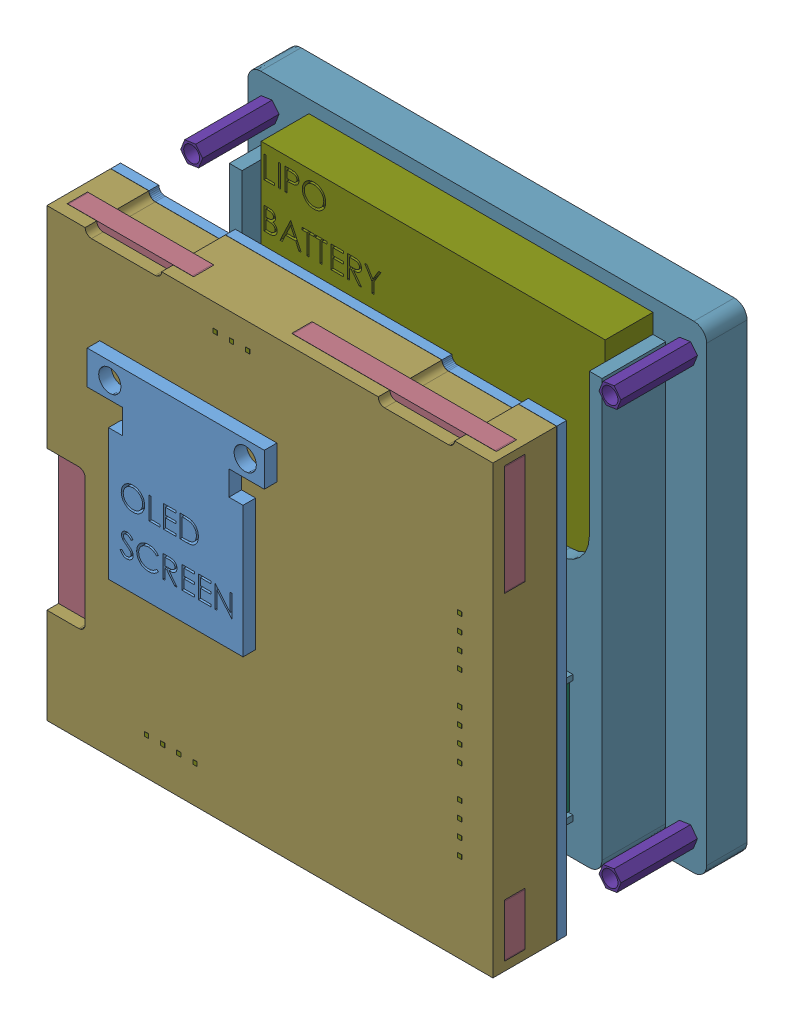
SolidWorks assembly IoTracking_PCB_Mech, configuration Default. Lengths in mm. (continued)
Components (placement in the parent): (continued)
- IoTracking_PCBboard-1: IoTracking_PCBboard [Default] at origin size (70 70 13.59) (continued)
  - IoTracking_PCB_new.step-1: IoTracking_PCB_new.step [Default] at origin size (70.02 70.02 13.59) (continued)
    - R3.step-1: R3.step [Default] at origin size (0.95 1.65 0.5) (continued)
      - 6125954208.step-1: 6125954208.step [Default] at (4.826 47.665 0) size (0.95 0.3 0.5)
        - Extruded-19.step-1: Extruded-19.step [Default] at origin size (0.95 0.3 0.5)
      - 6125954208.step-2: 6125954208.step [Default] at (4.826 46.315 0) size (0.95 0.3 0.5)
        - Extruded-19.step-1: Extruded-19.step [Default] at origin size (0.95 0.3 0.5)
      - 6125954368.step-1: 6125954368.step [Default] at (4.826 46.99 0) size (0.95 1.05 0.5)
        - Extruded-18.step-1: Extruded-18.step [Default] at origin size (0.95 1.05 0.5)
    - R2.step-1: R2.step [Default] at origin size (0.95 1.7 0.6)
      - 6127426432.step-1: 6127426432.step [Default] at (15.1893 55.6857 0) size (0.95 0.27 0.6)
        - Extruded-13.step-1: Extruded-13.step [Default] at origin size (0.95 0.27 0.6)
      - 6127426272.step-1: 6127426272.step [Default] at (15.1893 56.4007 0) size (0.95 1.16 0.6)
        - Extruded-14.step-1: Extruded-14.step [Default] at origin size (0.95 1.16 0.6)
      - 6127426432.step-2: 6127426432.step [Default] at (15.1893 57.1157 0) size (0.95 0.27 0.6)
        - Extruded-13.step-1: Extruded-13.step [Default] at origin size (0.95 0.27 0.6)
    - R1.step-1: R1.step [Default] at origin size (0.95 1.7 0.6)
      - 6127426432.step-1: 6127426432.step [Default] at (11.4301 55.6729 0) size (0.95 0.27 0.6)
        - Extruded-13.step-1: Extruded-13.step [Default] at origin size (0.95 0.27 0.6)
      - 6127426272.step-1: 6127426272.step [Default] at (11.4301 56.3879 0) size (0.95 1.16 0.6)
        - Extruded-14.step-1: Extruded-14.step [Default] at origin size (0.95 1.16 0.6)
      - 6127426432.step-2: 6127426432.step [Default] at (11.4301 57.1029 0) size (0.95 0.27 0.6)
        - Extruded-13.step-1: Extruded-13.step [Default] at origin size (0.95 0.27 0.6)
    - P5.step-1: P5.step [Default] at origin size (10.16 5.72 13.59)
      - 6127411952.step-1: 6127411952.step [Default] at (20.7009 5.8419 -3.56) size (0.64 0.64 13.59)
        - Extruded-22.step-1: Extruded-22.step [Default] at origin size (0.64 0.64 13.59)
      - 6127411952.step-2: 6127411952.step [Default] at (18.1609 5.842 -3.56) size (0.64 0.64 13.59)
        - Extruded-22.step-1: Extruded-22.step [Default] at origin size (0.64 0.64 13.59)
      - 6127411952.step-3: 6127411952.step [Default] at (15.6209 5.8418 -3.56) size (0.64 0.64 13.59)
        - Extruded-22.step-1: Extruded-22.step [Default] at origin size (0.64 0.64 13.59)
      - 6127411952.step-4: 6127411952.step [Default] at (23.2409 5.8419 -3.56) size (0.64 0.64 13.59)
        - Extruded-22.step-1: Extruded-22.step [Default] at origin size (0.64 0.64 13.59)
      - 6125956208.step-1: 6125956208.step [Default] at (19.431 5.5245 0) size (10.16 5.71 2.54)
        - Extruded-23.step-1: Extruded-23.step [Default] at origin size (10.16 5.71 2.54)
      - 6125956048.step-1: 6125956048.step [Default] at (19.431 3.4265 2.54) size (7.62 1.53 5.33)
        - Extruded-24.step-1: Extruded-24.step [Default] at origin size (7.62 1.53 5.33)
    - P4.step-1: P4.step [Default] at origin size (5.72 10.16 13.59)
      - 6125954528.step-1: 6125954528.step [Default] at (62.3545 17.78 2.54) size (1.53 7.62 5.33)
        - Extruded-25.step-1: Extruded-25.step [Default] at origin size (1.53 7.62 5.33)
      - 6125954688.step-1: 6125954688.step [Default] at (64.4525 17.78 0) size (5.71 10.16 2.54)
        - Extruded-26.step-1: Extruded-26.step [Default] at origin size (5.71 10.16 2.54)
      - 6127411952.step-1: 6127411952.step [Default] at (64.7699 13.9701 -3.56) size (0.64 0.64 13.59)
        - Extruded-22.step-1: Extruded-22.step [Default] at origin size (0.64 0.64 13.59)
      - 6127411952.step-2: 6127411952.step [Default] at (64.7698 21.5901 -3.56) size (0.64 0.64 13.59)
        - Extruded-22.step-1: Extruded-22.step [Default] at origin size (0.64 0.64 13.59)
      - 6127411952.step-3: 6127411952.step [Default] at (64.7699 19.0501 -3.56) size (0.64 0.64 13.59)
        - Extruded-22.step-1: Extruded-22.step [Default] at origin size (0.64 0.64 13.59)
      - 6127411952.step-4: 6127411952.step [Default] at (64.7699 16.5101 -3.56) size (0.64 0.64 13.59)
        - Extruded-22.step-1: Extruded-22.step [Default] at origin size (0.64 0.64 13.59)
    - P3.step-1: P3.step [Default] at origin size (5.72 10.16 13.59)
      - 6127411952.step-1: 6127411952.step [Default] at (64.7699 29.2101 -3.56) size (0.64 0.64 13.59)
        - Extruded-22.step-1: Extruded-22.step [Default] at origin size (0.64 0.64 13.59)
      - 6127411952.step-2: 6127411952.step [Default] at (64.7699 31.7501 -3.56) size (0.64 0.64 13.59)
        - Extruded-22.step-1: Extruded-22.step [Default] at origin size (0.64 0.64 13.59)
      - 6127411952.step-3: 6127411952.step [Default] at (64.7698 34.2901 -3.56) size (0.64 0.64 13.59)
        - Extruded-22.step-1: Extruded-22.step [Default] at origin size (0.64 0.64 13.59)
      - 6127411952.step-4: 6127411952.step [Default] at (64.7699 26.6701 -3.56) size (0.64 0.64 13.59)
        - Extruded-22.step-1: Extruded-22.step [Default] at origin size (0.64 0.64 13.59)
      - 6125954688.step-1: 6125954688.step [Default] at (64.4525 30.48 0) size (5.71 10.16 2.54)
        - Extruded-26.step-1: Extruded-26.step [Default] at origin size (5.71 10.16 2.54)
      - 6125954528.step-1: 6125954528.step [Default] at (62.3545 30.48 2.54) size (1.53 7.62 5.33)
        - Extruded-25.step-1: Extruded-25.step [Default] at origin size (1.53 7.62 5.33)
    - P2.step-1: P2.step [Default] at origin size (5.72 10.16 13.59)
      - 6125954528.step-1: 6125954528.step [Default] at (62.3545 43.18 2.54) size (1.53 7.62 5.33)
        - Extruded-25.step-1: Extruded-25.step [Default] at origin size (1.53 7.62 5.33)
      - 6125954688.step-1: 6125954688.step [Default] at (64.4525 43.18 0) size (5.71 10.16 2.54)
        - Extruded-26.step-1: Extruded-26.step [Default] at origin size (5.71 10.16 2.54)
      - 6127411952.step-1: 6127411952.step [Default] at (64.7699 39.3701 -3.56) size (0.64 0.64 13.59)
        - Extruded-22.step-1: Extruded-22.step [Default] at origin size (0.64 0.64 13.59)
      - 6127411952.step-2: 6127411952.step [Default] at (64.7698 46.9901 -3.56) size (0.64 0.64 13.59)
        - Extruded-22.step-1: Extruded-22.step [Default] at origin size (0.64 0.64 13.59)
      - 6127411952.step-3: 6127411952.step [Default] at (64.7699 44.4501 -3.56) size (0.64 0.64 13.59)
        - Extruded-22.step-1: Extruded-22.step [Default] at origin size (0.64 0.64 13.59)
      - 6127411952.step-4: 6127411952.step [Default] at (64.7699 41.9101 -3.56) size (0.64 0.64 13.59)
        - Extruded-22.step-1: Extruded-22.step [Default] at origin size (0.64 0.64 13.59)
    - P1.step-1: P1.step [Default] at origin size (7.62 5.72 13.59)
      - 6127411472.step-1: 6127411472.step [Default] at (28.956 63.627 2.54) size (5.08 1.52 5.33)
        - Extruded-27.step-1: Extruded-27.step [Default] at origin size (5.08 1.52 5.33)
      - 6127411632.step-1: 6127411632.step [Default] at (28.956 65.7225 0) size (7.62 5.71 2.54)
        - Extruded-28.step-1: Extruded-28.step [Default] at origin size (7.62 5.71 2.54)
      - 6127411952.step-1: 6127411952.step [Default] at (31.4959 66.0399 -3.56) size (0.64 0.64 13.59)
        - Extruded-22.step-1: Extruded-22.step [Default] at origin size (0.64 0.64 13.59)
      - 6127411952.step-2: 6127411952.step [Default] at (26.4159 66.0399 -3.56) size (0.64 0.64 13.59)
        - Extruded-22.step-1: Extruded-22.step [Default] at origin size (0.64 0.64 13.59)
      - 6127411952.step-3: 6127411952.step [Default] at (28.9559 66.0399 -3.56) size (0.64 0.64 13.59)
        - Extruded-22.step-1: Extruded-22.step [Default] at origin size (0.64 0.64 13.59)
    - L_B1.step-1: L_B1.step [Default] at origin size (7.01 6.9 4)
      - 744311220.step-1: 744311220.step [Default] at (43.434 52.07 1.6) x (0 1 0) z (0 0 1) size (6.9 7.01 4)
        - Geh_use.step-1: Geh_use.step [Default] at origin size (6.9 6.9 2.4)
        - Spule.step-1: Spule.step [Default] at (0 0 -0.0088) x (0 -1 0) z (0 0 1) size (7.01 5.89 3.39)
        - Boden.step-1: Boden.step [Default] at (0 0 -1.5) size (6.9 6.9 1.5)
        - Klebemasse.step-1: Klebemasse.step [Default] at (0 3.25 0) x (-1 0 0) z (0 0 1) size (3.5 0.4 3.8)
        - Klebemasse.step-2: Klebemasse.step [Default] at (0 -3.25 0) size (3.5 0.4 3.8)
    - J1.step-1: J1.step [Default] at origin size (8.8 5.73 2.94)
      - ZX62R-B-5P.step-1: ZX62R-B-5P.step [Default] at (13.238 63.2505 0) x (-1 0 0) z (0 1 0) size (8.8 2.94 5.73)
    - FB1.step-1: FB1.step [Default] at origin size (1.25 2 1.05)
      - FBead_Murata_BLM21AG102SN1D_eec.step-1: FBead_Murata_BLM21AG102SN1D_eec.step [Default] at (6.858 59.69 0) x (0 1 0) z (0 0 1) size (2 1.25 1.05)
        - Electrodes.step-1: Electrodes.step [Default] at origin size (2 1.25 1.05)
        - Dielectric.step-1: Dielectric.step [Default] at origin size (1 1.24 1.04)
        - Murata.step-1: Murata.step [Default] at origin size (0.53 0.12 0)
    - DS1.step-1: DS1.step [Default] at origin size (0.8 1.6 0.65)
      - Diode_Lite-On_LTST-C191KGKT_eec.step-1: Diode_Lite-On_LTST-C191KGKT_eec.step [Default] at (27.0764 14.732 0) x (0 -1 0) z (0 0 1) size (1.6 0.8 0.65)
        - 1-29.step-1: 1-29.step [Default] at origin size (1.6 0.8 0.16)
        - 2-30.step-1: 2-30.step [Default] at origin size (1.1 0.8 0.47)
        - 3-31.step-1: 3-31.step [Default] at origin size (1.6 0.7 0.18)
        - Lite-On_Logo_Adjustable.step-1: Lite-On_Logo_Adjustable.step [Default] at (-0.9403 -0.3001 -1.9063) x (1 0 0) z (0 -1 0) size (0.21 0.05 0.1)
    - D4.step-1: D4.step [Default] at origin size (1.25 2 1.2)
      - Diode_Lite-On_LTST-C170GKT_eec.step-1: Diode_Lite-On_LTST-C170GKT_eec.step [Default] at (22.606 56.642 0) x (1 0 0) z (0 0 1) size (1.25 2 1.2)
        - 1-32.step-1: 1-32.step [Default] at origin size (0.15 0.15 0.05)
        - 2-33.step-1: 2-33.step [Default] at origin size (1.25 2 0.5)
        - 3-34.step-1: 3-34.step [Default] at origin size (1.25 1.4 0.75)
        - 4-35.step-1: 4-35.step [Default] at origin size (1.25 1.9 0.4)
        - Lite-On_Logo_Adjustable-36.step-1: Lite-On_Logo_Adjustable-36.step [Default] at (0.526 -1.0018 -1.9007) x (0 1 0) z (1 0 0) size (0.43 0.1 0.1)
        - 5-37.step-1: 5-37.step [Default] at origin size (1.25 0.3 0.03)
    - D3.step-1: D3.step [Default] at origin size (1.25 2 1.2)
      - Diode_Lite-On_LTST-C170CKT_eec.step-1: Diode_Lite-On_LTST-C170CKT_eec.step [Default] at (22.606 51.816 0) x (0 -1 0) z (0 0 1) size (2 1.25 1.2)
        - pcb.step-1: pcb.step [Default] at (0 0 0.01) size (1.98 1.25 0.48)
        - top.step-1: top.step [Default] at (0 0 0.49) size (1.4 1.25 0.71)
        - lead.step-1: lead.step [Default] at (-0.7501 0 0.5) x (-1 0 0) z (0 0 -1) size (0.5 1.25 0.5)
        - emitter.step-1: emitter.step [Default] at (-0.0551 -0.005 1.2) size (0.15 0.15 0)
        - lead_MIR1.step-1: lead_MIR1.step [Default] at (0.7499 0 0.5) size (0.5 1.25 0.5)
        - marking.step-1: marking.step [Default] at (-0.9399 0 0.5) size (0.31 1.25 0)
    - D2.step-1: D2.step [Default] at origin size (1.4 3 1.1)
      - 6127411312.step-1: 6127411312.step [Default] at (12.573 60.198 0) size (1.4 3 1.1)
        - Extruded-38.step-1: Extruded-38.step [Default] at origin size (1.4 3 1.1)
    - D1.step-1: D1.step [Default] at origin size (2 1.25 1.2)
      - Diode_Lite-On_LTST-C170CKT_eec.step-1: Diode_Lite-On_LTST-C170CKT_eec.step [Default] at (10.086 45.6292 0) x (-1 0 0) z (0 0 1) size (2 1.25 1.2)
        - pcb.step-1: pcb.step [Default] at (0 0 0.01) size (1.98 1.25 0.48)
        - top.step-1: top.step [Default] at (0 0 0.49) size (1.4 1.25 0.71)
        - lead.step-1: lead.step [Default] at (-0.7501 0 0.5) x (-1 0 0) z (0 0 -1) size (0.5 1.25 0.5)
        - emitter.step-1: emitter.step [Default] at (-0.0551 -0.005 1.2) size (0.15 0.15 0)
        - lead_MIR1.step-1: lead_MIR1.step [Default] at (0.7499 0 0.5) size (0.5 1.25 0.5)
        - marking.step-1: marking.step [Default] at (-0.9399 0 0.5) size (0.31 1.25 0)
    - C_B2.step-1: C_B2.step [Default] at origin size (2.01 2.72 1.43)
      - Cap_TDK_Corporation_C1608X5R1C106M080AB_eec.step-1: Cap_TDK_Corporation_C1608X5R1C106M080AB_eec.step [Default] at (40.259 45.782 0) x (0 -1 0) z (0 0 1) size (2.72 2.01 1.43)
        - body.step-1: body.step [Default] at origin size (1.2 0.8 0.8)
        - Terminals.step-1: Terminals.step [Default] at (0.6 -0.4 0) x (0 1 0) z (1 0 0) size (2.01 1.25 1.52)
        - value.step-1: value.step [Default] at (0 0 0.8) size (0.79 0.68 0.25)
    - C_B1.step-1: C_B1.step [Default] at origin size (0.9 1.7 1)
      - 6125950048.step-1: 6125950048.step [Default] at (44.704 45.632 0) size (0.9 1.3 1)
        - Extruded-39.step-1: Extruded-39.step [Default] at origin size (0.9 1.3 1)
      - 6125949888.step-1: 6125949888.step [Default] at (44.704 44.882 0) size (0.9 0.2 1)
        - Extruded-40.step-1: Extruded-40.step [Default] at origin size (0.9 0.2 1)
      - 6125949888.step-2: 6125949888.step [Default] at (44.704 46.382 0) size (0.9 0.2 1)
        - Extruded-40.step-1: Extruded-40.step [Default] at origin size (0.9 0.2 1)
    - C_A2.step-1: C_A2.step [Default] at origin size (0.3 0.6 0.34)
      - Cap_Murata_GRM0335C1HR30BA01D_eec.step-1: Cap_Murata_GRM0335C1HR30BA01D_eec.step [Default] at (18.542 39.37 0) x (0 1 0) z (0 0 1) size (0.6 0.3 0.34)
        - terminals-41.step-1: terminals-41.step [Default] at origin size (0.6 0.3 0.33)
        - body-42.step-1: body-42.step [Default] at origin size (0.3 0.3 0.33)
        - logo.step-1: logo.step [Default] at (-0.2332 0.5956 0.33) size (0.25 0.06 0.01)
    - C_A1.step-1: C_A1.step [Default] at origin size (0.3 0.6 0.34)
      - Cap_Murata_GRM0335C1HR30BA01D_eec.step-1: Cap_Murata_GRM0335C1HR30BA01D_eec.step [Default] at (18.542 42.672 0) x (0 1 0) z (0 0 1) size (0.6 0.3 0.34)
        - terminals-41.step-1: terminals-41.step [Default] at origin size (0.6 0.3 0.33)
        - body-42.step-1: body-42.step [Default] at origin size (0.3 0.3 0.33)
        - logo.step-1: logo.step [Default] at (-0.2332 0.5956 0.33) size (0.25 0.06 0.01)
    - C16.step-1: C16.step [Default] at origin size (2.2 1.45 1.45)
      - 6127425232.step-1: 6127425232.step [Default] at (27.99 60.96 0) size (0.5 1.45 1.45)
        - Extruded-43.step-1: Extruded-43.step [Default] at origin size (0.5 1.45 1.45)
      - 6127425232.step-2: 6127425232.step [Default] at (29.69 60.96 0) size (0.5 1.45 1.45)
        - Extruded-43.step-1: Extruded-43.step [Default] at origin size (0.5 1.45 1.45)
      - 6127425392.step-1: 6127425392.step [Default] at (28.84 60.96 0) size (1.2 1.45 1.45)
        - Extruded-44.step-1: Extruded-44.step [Default] at origin size (1.2 1.45 1.45)
    - C15.step-1: C15.step [Default] at origin size (1.45 2.2 1.45)
      - 6125947888.step-1: 6125947888.step [Default] at (25.654 50.634 0) size (1.45 0.5 1.45)
        - Extruded-45.step-1: Extruded-45.step [Default] at origin size (1.45 0.5 1.45)
      - 6125947888.step-2: 6125947888.step [Default] at (25.654 48.934 0) size (1.45 0.5 1.45)
        - Extruded-45.step-1: Extruded-45.step [Default] at origin size (1.45 0.5 1.45)
      - 6125947648.step-1: 6125947648.step [Default] at (25.654 49.784 0) size (1.45 1.2 1.45)
        - Extruded-46.step-1: Extruded-46.step [Default] at origin size (1.45 1.2 1.45)
    - C14.step-1: C14.step [Default] at origin size (0.96 1.75 0.9)
      - 6125952448.step-1: 6125952448.step [Default] at (20.066 59.944 0) size (0.96 1.05 0.9)
        - Extruded-47.step-1: Extruded-47.step [Default] at origin size (0.96 1.05 0.9)
      - 6125952288.step-1: 6125952288.step [Default] at (20.066 59.244 0) size (0.96 0.35 0.9)
        - Extruded-48.step-1: Extruded-48.step [Default] at origin size (0.96 0.35 0.9)
      - 6125952288.step-2: 6125952288.step [Default] at (20.066 60.644 0) size (0.96 0.35 0.9)
        - Extruded-48.step-1: Extruded-48.step [Default] at origin size (0.96 0.35 0.9)
    - C13.step-1: C13.step [Default] at origin size (1.75 0.95 0.95)
      - 6125953728.step-1: 6125953728.step [Default] at (49.276 66.04 0) size (0.95 0.95 0.95)
        - Extruded.step-1: Extruded.step [Default] at origin size (0.95 0.95 0.95)
      - 6125949568.step-1: 6125949568.step [Default] at (49.951 66.04 0) size (0.4 0.95 0.95)
        - Extruded-49.step-1: Extruded-49.step [Default] at origin size (0.4 0.95 0.95)
      - 6125949568.step-2: 6125949568.step [Default] at (48.601 66.04 0) size (0.4 0.95 0.95)
        - Extruded-49.step-1: Extruded-49.step [Default] at origin size (0.4 0.95 0.95)
    - C12.step-1: C12.step [Default] at origin size (0.95 1.75 1)
      - 6127425632.step-1: 6127425632.step [Default] at (36.068 31.304 0) size (0.95 0.35 1)
        - Extruded-50.step-1: Extruded-50.step [Default] at origin size (0.95 0.35 1)
      - 6127425632.step-2: 6127425632.step [Default] at (36.068 32.704 0) size (0.95 0.35 1)
        - Extruded-50.step-1: Extruded-50.step [Default] at origin size (0.95 0.35 1)
      - 6127425792.step-1: 6127425792.step [Default] at (36.068 32.004 0) size (0.95 1.05 1)
        - Extruded-51.step-1: Extruded-51.step [Default] at origin size (0.95 1.05 1)
    - C11.step-1: C11.step [Default] at origin size (0.95 1.75 1)
      - 6127425632.step-1: 6127425632.step [Default] at (36.0934 29.529 0) size (0.95 0.35 1)
        - Extruded-50.step-1: Extruded-50.step [Default] at origin size (0.95 0.35 1)
      - 6127425632.step-2: 6127425632.step [Default] at (36.0934 28.129 0) size (0.95 0.35 1)
        - Extruded-50.step-1: Extruded-50.step [Default] at origin size (0.95 0.35 1)
      - 6127425792.step-1: 6127425792.step [Default] at (36.0934 28.829 0) size (0.95 1.05 1)
        - Extruded-51.step-1: Extruded-51.step [Default] at origin size (0.95 1.05 1)
    - C10.step-1: C10.step [Default] at origin size (0.96 1.75 0.9)
      - 6125952448.step-1: 6125952448.step [Default] at (33.02 10.9728 0) size (0.96 1.05 0.9)
        - Extruded-47.step-1: Extruded-47.step [Default] at origin size (0.96 1.05 0.9)
      - 6125952288.step-1: 6125952288.step [Default] at (33.02 10.2728 0) size (0.96 0.35 0.9)
        - Extruded-48.step-1: Extruded-48.step [Default] at origin size (0.96 0.35 0.9)
      - 6125952288.step-2: 6125952288.step [Default] at (33.02 11.6728 0) size (0.96 0.35 0.9)
        - Extruded-48.step-1: Extruded-48.step [Default] at origin size (0.96 0.35 0.9)
    - C8.step-1: C8.step [Default] at origin size (2.01 1.25 1.52)
      - Cap_AVX_0805YA103FAT2A_eec.step-1: Cap_AVX_0805YA103FAT2A_eec.step [Default] at (15.24 17.018 0) x (-1 0 0) z (0 0 1) size (2.01 1.25 1.52)
        - Terminals.step-1: Terminals.step [Default] at origin size (2.01 1.25 1.52)
        - Electrode.step-1: Electrode.step [Default] at origin size (1.01 1.25 1.52)
        - AVX.step-1: AVX.step [Default] at origin size (0.37 0.13 0)
    - C7.step-1: C7.step [Default] at origin size (1.75 0.95 0.95)
      - 6125953728.step-1: 6125953728.step [Default] at (7.874 50.292 0) size (0.95 0.95 0.95)
        - Extruded.step-1: Extruded.step [Default] at origin size (0.95 0.95 0.95)
      - 6125949568.step-1: 6125949568.step [Default] at (7.199 50.292 0) size (0.4 0.95 0.95)
        - Extruded-49.step-1: Extruded-49.step [Default] at origin size (0.4 0.95 0.95)
      - 6125949568.step-2: 6125949568.step [Default] at (8.549 50.292 0) size (0.4 0.95 0.95)
        - Extruded-49.step-1: Extruded-49.step [Default] at origin size (0.4 0.95 0.95)
    - C6.step-1: C6.step [Default] at origin size (0.95 1.75 1)
      - 6127425632.step-1: 6127425632.step [Default] at (16.9672 57.1008 0) size (0.95 0.35 1)
        - Extruded-50.step-1: Extruded-50.step [Default] at origin size (0.95 0.35 1)
      - 6127425632.step-2: 6127425632.step [Default] at (16.9672 55.7008 0) size (0.95 0.35 1)
        - Extruded-50.step-1: Extruded-50.step [Default] at origin size (0.95 0.35 1)
      - 6127425792.step-1: 6127425792.step [Default] at (16.9672 56.4008 0) size (0.95 1.05 1)
        - Extruded-51.step-1: Extruded-51.step [Default] at origin size (0.95 1.05 1)
    - C5.step-1: C5.step [Default] at origin size (0.95 1.75 1)
      - 6127425632.step-1: 6127425632.step [Default] at (9.652 57.088 0) size (0.95 0.35 1)
        - Extruded-50.step-1: Extruded-50.step [Default] at origin size (0.95 0.35 1)
      - 6127425632.step-2: 6127425632.step [Default] at (9.652 55.688 0) size (0.95 0.35 1)
        - Extruded-50.step-1: Extruded-50.step [Default] at origin size (0.95 0.35 1)
      - 6127425792.step-1: 6127425792.step [Default] at (9.652 56.388 0) size (0.95 1.05 1)
        - Extruded-51.step-1: Extruded-51.step [Default] at origin size (0.95 1.05 1)
    - C4.step-1: C4.step [Default] at origin size (1.45 2.2 1.45)
      - 6125947888.step-1: 6125947888.step [Default] at (4.826 62.904 0) size (1.45 0.5 1.45)
        - Extruded-45.step-1: Extruded-45.step [Default] at origin size (1.45 0.5 1.45)
      - 6125947888.step-2: 6125947888.step [Default] at (4.826 64.604 0) size (1.45 0.5 1.45)
        - Extruded-45.step-1: Extruded-45.step [Default] at origin size (1.45 0.5 1.45)
      - 6125947648.step-1: 6125947648.step [Default] at (4.826 63.754 0) size (1.45 1.2 1.45)
        - Extruded-46.step-1: Extruded-46.step [Default] at origin size (1.45 1.2 1.45)
    - C2.step-1: C2.step [Default] at origin size (0.95 1.75 0.87)
      - 6125945248.step-1: 6125945248.step [Default] at (9.652 60.198 0) size (0.95 1.05 0.87)
        - Extruded-52.step-1: Extruded-52.step [Default] at origin size (0.95 1.05 0.87)
      - 6125945088.step-1: 6125945088.step [Default] at (9.652 60.898 0) size (0.95 0.35 0.87)
        - Extruded-53.step-1: Extruded-53.step [Default] at origin size (0.95 0.35 0.87)
      - 6125945088.step-2: 6125945088.step [Default] at (9.652 59.498 0) size (0.95 0.35 0.87)
        - Extruded-53.step-1: Extruded-53.step [Default] at origin size (0.95 0.35 0.87)
    - C1.step-1: C1.step [Default] at origin size (1.75 0.95 0.95)
      - 6125953728.step-1: 6125953728.step [Default] at (7.874 53.34 0) size (0.95 0.95 0.95)
        - Extruded.step-1: Extruded.step [Default] at origin size (0.95 0.95 0.95)
      - 6125949568.step-1: 6125949568.step [Default] at (7.199 53.34 0) size (0.4 0.95 0.95)
        - Extruded-49.step-1: Extruded-49.step [Default] at origin size (0.4 0.95 0.95)
      - 6125949568.step-2: 6125949568.step [Default] at (8.549 53.34 0) size (0.4 0.95 0.95)
        - Extruded-49.step-1: Extruded-49.step [Default] at origin size (0.4 0.95 0.95)
    - Free-Models.step-1: Free-Models.step [Default] at origin size (70 70 10)
      - boardSmall.step-1: boardSmall.step [Default] at (34.977 34.9758 0) size (70 70 10) (hidden)
- transparent_cover_1_8in-3: transparent_cover_1_8in [Default] at (34.999 34.999 5) size (70 70 3.17)
- 3dprint_bottombox-3: 3dprint_bottombox [Default] at (34.989 34.989 -28.8842) size (72 75 24.85)
- gps_dummy-4: gps_dummy [Default] at (50.489 15.139 -12.5342) x (0 -1 0) z (0 0 1) size (18 18 7.1)
- lipobat_dummy-4: lipobat_dummy [Default] at (35.569 36.489 -22.5342) x (0 1 0) z (0 0 1) size (68 54 7.5)
- m2_5_standoff_long-5: m2_5_standoff_long [Default] at (2.159 2.159 -22.5342) size (3.46 3.26 12)
- m2_5_standoff_long-6: m2_5_standoff_long [Default] at (2.159 67.819 -22.5342) size (3.46 3.26 12)
- m2_5_standoff_long-7: m2_5_standoff_long [Default] at (67.819 67.819 -22.5342) size (3.46 3.26 12)
- m2_5_standoff_long-8: m2_5_standoff_long [Default] at (67.819 2.159 -22.5342) size (3.46 3.26 12)
- m2_5_standoff-5: m2_5_standoff [Default] at (2.159 67.818 0) x (-0.732098 -0.681199 0) z (0 0 1) size (3.46 3.26 5)
- m2_5_standoff-6: m2_5_standoff [Default] at (2.159 2.159 0) x (-0.732098 -0.681199 0) z (0 0 1) size (3.46 3.26 5)
- m2_5_standoff-7: m2_5_standoff [Default] at (67.818 67.818 0) x (-0.732098 -0.681199 0) z (0 0 1) size (3.46 3.26 5)
- m2_5_standoff-8: m2_5_standoff [Default] at (67.818 2.159 0) x (-0.732098 -0.681199 0) z (0 0 1) size (3.46 3.26 5)
- oled_dummy-3: oled_dummy [Default] at (22.175 55.7456 11.975) x (-1 0 0) z (0 0 -1) size (27.8 29.76 6.8)
Mates (geometry in assembly coordinates):
- Coincident1: coincident: point of IoTracking_PCBboard-1/IoTracking_PCB_new.step-1/Board.step-1/Open CASCADE STEP translator 6.8 1.1.1.step-1
- Coincident2: coincident aligned: plane of IoTracking_PCBboard-1/IoTracking_PCB_new.step-1/Board.step-1/Open CASCADE STEP translator 6.8 1.1.1.step-1 through (70 70 0) normal (0 0 1)
- Coincident3: coincident anti-aligned: plane of IoTracking_PCBboard-1/IoTracking_PCB_new.step-1/Board.step-1/Open CASCADE STEP translator 6.8 1.1.1.step-1 through (0 15 -1.5342) normal (-1 0 0)
- Concentric1: concentric aligned: cylinder of IoTracking_PCBboard-1/IoTracking_PCB_new.step-1/Board.step-1/Open CASCADE STEP translator 6.8 1.1.1.step-1 through (2.159 67.818 -1.5342) axis (0 0 -1) radius 1.35; cylinder of transparent_cover_1_8in-3 through (2.159 67.819 8.175) axis (0 0 -1) radius 1.35
- Concentric2: concentric aligned: cylinder of IoTracking_PCBboard-1/IoTracking_PCB_new.step-1/Board.step-1/Open CASCADE STEP translator 6.8 1.1.1.step-1 through (2.159 2.159 -1.5342) axis (0 0 -1) radius 1.35; cylinder of transparent_cover_1_8in-3 through (2.159 2.159 8.175) axis (0 0 -1) radius 1.35
- Distance1: distance = 5 mm anti-aligned: plane of transparent_cover_1_8in-3 through (34.999 34.999 5) normal (0 0 -1); plane of IoTracking_PCBboard-1/IoTracking_PCB_new.step-1/Board.step-1/Open CASCADE STEP translator 6.8 1.1.1.step-1 through (70 70 0) normal (0 0 1)
- Distance4: distance = 2.5 mm anti-aligned: plane of 3dprint_bottombox-3 through (34.989 34.989 -4.0342) normal (0 0 1); plane of IoTracking_PCBboard-1/IoTracking_PCB_new.step-1/Board.step-1/Open CASCADE STEP translator 6.8 1.1.1.step-1 through (70 70 -1.5342) normal (0 0 -1)
- Concentric18: concentric aligned: cylinder of transparent_cover_1_8in-3 through (2.159 2.159 8.175) axis (0 0 -1) radius 1.35; cylinder of 3dprint_bottombox-3 through (2.159 2.159 -22.5342) axis (0 0 -1) radius 1.35
- Concentric19: concentric aligned: cylinder of transparent_cover_1_8in-3 through (67.819 2.159 8.175) axis (0 0 -1) radius 1.35; cylinder of 3dprint_bottombox-3 through (67.819 2.159 -22.5342) axis (0 0 -1) radius 1.35
- Coincident16: coincident anti-aligned: plane of 3dprint_bottombox-3 through (41.489 34.989 -28.8842) normal (1 0 0); plane of gps_dummy-4 through (41.489 24.139 -5.4342) normal (-1 0 0)
- Coincident17: coincident anti-aligned: plane of 3dprint_bottombox-3 through (41.489 24.139 -12.5342) normal (0 -1 0); plane of gps_dummy-4 through (59.489 24.139 -5.4342) normal (0 1 0)
- Coincident18: coincident anti-aligned: plane of 3dprint_bottombox-3 through (34.989 34.989 -12.5342) normal (0 0 1); plane of gps_dummy-4 through (50.489 15.139 -12.5342) normal (0 0 -1)
- Coincident19: coincident anti-aligned: plane of 3dprint_bottombox-3 through (62.569 34.989 -12.5342) normal (-1 0 0); plane of lipobat_dummy-4 through (62.569 2.489 -15.0342) normal (1 0 0)
- Coincident20: coincident anti-aligned: plane of 3dprint_bottombox-3 through (34.989 2.489 -12.5342) normal (0 1 0); plane of lipobat_dummy-4 through (8.569 2.489 -15.0342) normal (0 -1 0)
- Coincident21: coincident anti-aligned: plane of 3dprint_bottombox-3 through (34.989 34.989 -22.5342) normal (0 0 1); plane of lipobat_dummy-4 through (35.569 36.489 -22.5342) normal (0 0 -1)
- Concentric20: concentric aligned: cylinder of 3dprint_bottombox-3 through (2.159 2.159 -22.5342) axis (0 0 -1) radius 1.35; cylinder of m2_5_standoff_long-5 through (2.159 2.159 -10.5342) axis (0 0 -1) radius 1.25
- Coincident22: coincident anti-aligned: plane of 3dprint_bottombox-3 through (34.989 34.989 -22.5342) normal (0 0 1); plane of m2_5_standoff_long-5 through (2.159 2.159 -22.5342) normal (0 0 -1)
- Concentric21: concentric aligned: cylinder of 3dprint_bottombox-3 through (67.819 2.159 -22.5342) axis (0 0 -1) radius 1.35; cylinder of m2_5_standoff_long-8 through (67.819 2.159 -10.5342) axis (0 0 -1) radius 1.25
- Concentric22: concentric aligned: cylinder of 3dprint_bottombox-3 through (2.159 67.819 -22.5342) axis (0 0 -1) radius 1.35; cylinder of m2_5_standoff_long-6 through (2.159 67.819 -10.5342) axis (0 0 -1) radius 1.25
- Concentric23: concentric aligned: cylinder of 3dprint_bottombox-3 through (67.819 67.819 -22.5342) axis (0 0 -1) radius 1.35; cylinder of m2_5_standoff_long-7 through (67.819 67.819 -10.5342) axis (0 0 -1) radius 1.25
- Coincident23: coincident anti-aligned: plane of 3dprint_bottombox-3 through (34.989 34.989 -22.5342) normal (0 0 1); plane of m2_5_standoff_long-7 through (67.819 67.819 -22.5342) normal (0 0 -1)
- Coincident24: coincident anti-aligned: plane of 3dprint_bottombox-3 through (34.989 34.989 -22.5342) normal (0 0 1); plane of m2_5_standoff_long-8 through (67.819 2.159 -22.5342) normal (0 0 -1)
- Coincident25: coincident anti-aligned: plane of 3dprint_bottombox-3 through (34.989 34.989 -22.5342) normal (0 0 1); plane of m2_5_standoff_long-6 through (2.159 67.819 -22.5342) normal (0 0 -1)
- Concentric24: concentric aligned: cylinder of IoTracking_PCBboard-1/IoTracking_PCB_new.step-1/Board.step-1/Open CASCADE STEP translator 6.8 1.1.1.step-1 through (2.159 67.818 -1.5342) axis (0 0 -1) radius 1.35; cylinder of m2_5_standoff-5 through (2.159 67.818 5) axis (0 0 -1) radius 1.25
- Coincident26: coincident anti-aligned: plane of IoTracking_PCBboard-1/IoTracking_PCB_new.step-1/Board.step-1/Open CASCADE STEP translator 6.8 1.1.1.step-1 through (70 70 0) normal (0 0 1); plane of m2_5_standoff-5 through (2.159 67.818 0) normal (0 0 -1)
- Concentric25: concentric aligned: cylinder of IoTracking_PCBboard-1/IoTracking_PCB_new.step-1/Board.step-1/Open CASCADE STEP translator 6.8 1.1.1.step-1 through (2.159 2.159 -1.5342) axis (0 0 -1) radius 1.35; cylinder of m2_5_standoff-6 through (2.159 2.159 5) axis (0 0 -1) radius 1.25
- Concentric26: concentric aligned: cylinder of IoTracking_PCBboard-1/IoTracking_PCB_new.step-1/Board.step-1/Open CASCADE STEP translator 6.8 1.1.1.step-1 through (67.818 2.159 -1.5342) axis (0 0 -1) radius 1.35; cylinder of m2_5_standoff-8 through (67.818 2.159 5) axis (0 0 -1) radius 1.25
- Concentric27: concentric aligned: cylinder of IoTracking_PCBboard-1/IoTracking_PCB_new.step-1/Board.step-1/Open CASCADE STEP translator 6.8 1.1.1.step-1 through (67.818 67.818 -1.5342) axis (0 0 -1) radius 1.35; cylinder of m2_5_standoff-7 through (67.818 67.818 5) axis (0 0 -1) radius 1.25
- Coincident28: coincident anti-aligned: plane of IoTracking_PCBboard-1/IoTracking_PCB_new.step-1/Board.step-1/Open CASCADE STEP translator 6.8 1.1.1.step-1 through (70 70 0) normal (0 0 1); plane of m2_5_standoff-8 through (67.818 2.159 0) normal (0 0 -1)
- Coincident29: coincident anti-aligned: plane of IoTracking_PCBboard-1/IoTracking_PCB_new.step-1/Board.step-1/Open CASCADE STEP translator 6.8 1.1.1.step-1 through (70 70 0) normal (0 0 1); plane of m2_5_standoff-7 through (67.818 67.818 0) normal (0 0 -1)
- Coincident30: coincident anti-aligned: plane of IoTracking_PCBboard-1/IoTracking_PCB_new.step-1/Board.step-1/Open CASCADE STEP translator 6.8 1.1.1.step-1 through (70 70 0) normal (0 0 1); plane of m2_5_standoff-6 through (2.159 2.159 0) normal (0 0 -1)
- Concentric30: concentric anti-aligned: cylinder of transparent_cover_1_8in-3 through (11.825 53.0956 8.175) axis (0 0 -1) radius 1.75; cylinder of oled_dummy-3 through (11.825 53.0956 8.175) axis (0 0 1) radius 1.75
- Concentric31: concentric anti-aligned: cylinder of transparent_cover_1_8in-3 through (33.075 53.0956 8.175) axis (0 0 -1) radius 1.75; cylinder of oled_dummy-3 through (33.075 53.0956 8.175) axis (0 0 1) radius 1.75
- Coincident33: coincident anti-aligned: plane of transparent_cover_1_8in-3 through (34.999 34.999 8.175) normal (0 0 1); plane of oled_dummy-3 through (22.175 55.7456 8.175) normal (0 0 -1)
